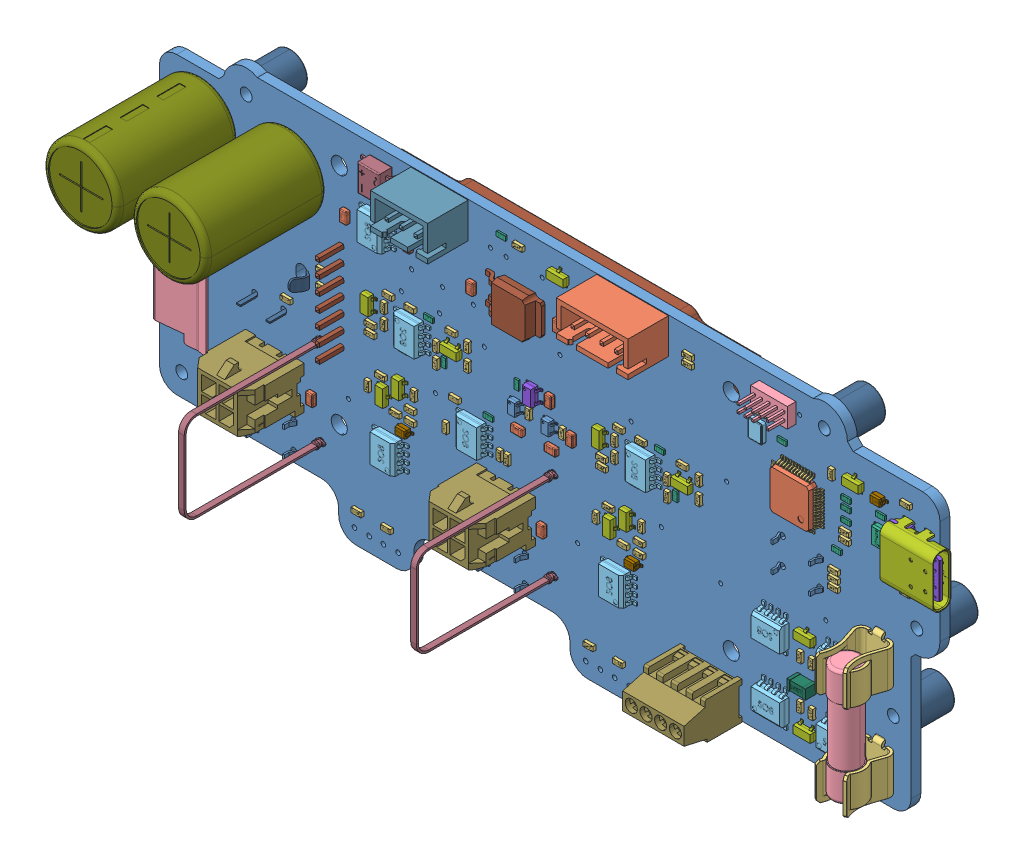
SolidWorks assembly SolderingStation, configuration Default. Lengths in mm.
Overall size (142.21 62 43.76).
390 component instances, 40 part files, 0 mates.
Components (placement in the parent):
- SolderingStation.step-1: SolderingStation.step [Default] at origin size (142.21 62 43.76)
  - Board_ss.step-1: Board_ss.step [Default] at origin size (140 62 1.69)
    - Open CASCADE STEP translator 6.8 4.1.1.step-1: Open CASCADE STEP translator 6.8 4.1.1.step [Default] at (0 0 -1.6914) size (140 62 1.69)
  - C17_ss.step-1: C17_ss.step [Default] at origin size (1.25 2 0.78)
    - User_Library-0805_SMD_Capacitor.step-1: User_Library-0805_SMD_Capacitor.step [Default] at (110.8455 64.7701 0) x (0 1 0) z (1 0 0) size (2 0.78 1.25)
  - R45_ss.step-1: R45_ss.step [Default] at origin size (1.7 0.8 0.56)
    - User_Library-RES_1609-0603.step-1: User_Library-RES_1609-0603.step [Default] at (65.2781 57.15 0) x (1 0 0) z (0 -1 0) size (1.7 0.56 0.8)
  - N1_ss.step-1: N1_ss.step [Default] at origin size (9.09 12.8 3.73)
    - nal-clip.step-1: nal-clip.step [Default] at (42.9877 48.2091 -0.8) x (0 0 -1) z (0 -1 0) size (3.73 9.09 12.8)
  - U2_ss.step-1: U2_ss.step [Default] at origin size (6.2 5 1.75)
    - User_Library-SOIC8_JEDEC_MS-012AA.step-1: User_Library-SOIC8_JEDEC_MS-012AA.step [Default] at (80.8676 75.6667 0) x (0 1 0) z (1 0 0) size (5 1.75 6.2)
  - C15_ss.step-1: C15_ss.step [Default] at origin size (1.6 0.8 0.3)
    - User_Library-0603_SMD_Capacitor.step-1: User_Library-0603_SMD_Capacitor.step [Default] at (161.9249 74.0409 0) x (-1 0 0) z (0 1 0) size (1.6 0.3 0.8)
  - C18_ss.step-1: C18_ss.step [Default] at origin size (1.6 0.8 0.3)
    - User_Library-0603_SMD_Capacitor.step-1: User_Library-0603_SMD_Capacitor.step [Default] at (161.9249 75.4379 0) x (-1 0 0) z (0 1 0) size (1.6 0.3 0.8)
  - U10_ss.step-1: U10_ss.step [Default] at origin size (3 2.5 1.1)
    - CircuitWorks-SOT-23.step-1: CircuitWorks-SOT-23.step [Default] at (163.4489 78.7147 0.5) x (-1 0 0) z (0 1 0) size (3 1.1 2.5)
  - U9_ss.step-1: U9_ss.step [Default] at origin size (2.8 2.9 1.45)
    - User_Library-SOT23-5-2.step-1: User_Library-SOT23-5-2.step [Default] at (107.9245 64.4143 0) x (0 -1 0) z (0 0 1) size (2.9 2.8 1.45)
  - C27_ss.step-1: C27_ss.step [Default] at origin size (1.25 2 0.78)
    - User_Library-0805_SMD_Capacitor.step-1: User_Library-0805_SMD_Capacitor.step [Default] at (114.5539 60.8331 0) x (0 1 0) z (1 0 0) size (2 0.78 1.25)
  - C26_ss.step-1: C26_ss.step [Default] at origin size (0.8 1.6 0.3)
    - User_Library-0603_SMD_Capacitor.step-1: User_Library-0603_SMD_Capacitor.step [Default] at (105.0035 64.1605 0) x (0 1 0) z (1 0 0) size (1.6 0.3 0.8)
  - C25_ss.step-1: C25_ss.step [Default] at origin size (1.25 2 0.78)
    - User_Library-0805_SMD_Capacitor.step-1: User_Library-0805_SMD_Capacitor.step [Default] at (109.4741 44.7039 0) x (0 -1 0) z (-1 0 0) size (2 0.78 1.25)
  - C24_ss.step-1: C24_ss.step [Default] at origin size (1.25 2 0.78)
    - User_Library-0805_SMD_Capacitor.step-1: User_Library-0805_SMD_Capacitor.step [Default] at (69.5961 44.4499 0) x (0 -1 0) z (-1 0 0) size (2 0.78 1.25)
  - D13_ss.step-1: D13_ss.step [Default] at origin size (2.7 1.25 1.1)
    - User_Library-SOD2513X11.step-1: User_Library-SOD2513X11.step [Default] at (167.7671 78.5115 0) x (1 0 0) z (0 0 1) size (2.7 1.25 1.1)
  - C22_ss.step-1: C22_ss.step [Default] at origin size (2 1.25 0.78)
    - User_Library-0805_SMD_Capacitor.step-1: User_Library-0805_SMD_Capacitor.step [Default] at (105.3871 57.6581 0) x (1 0 0) z (0 -1 0) size (2 0.78 1.25)
  - C23_ss.step-1: C23_ss.step [Default] at origin size (2 1.25 0.78)
    - User_Library-0805_SMD_Capacitor.step-1: User_Library-0805_SMD_Capacitor.step [Default] at (111.2291 57.6581 0) x (1 0 0) z (0 -1 0) size (2 0.78 1.25)
  - C21_ss.step-1: C21_ss.step [Default] at origin size (1.6 0.8 0.3)
    - User_Library-0603_SMD_Capacitor.step-1: User_Library-0603_SMD_Capacitor.step [Default] at (102.3367 85.0901 0) x (1 0 0) z (0 -1 0) size (1.6 0.3 0.8)
  - SP6_ss.step-1: SP6_ss.step [Default] at origin size (6 6 6)
    - 6mmSpacer.step-1: 6mmSpacer.step [Default] at (46.8629 36.8301 -1.6914) x (-1 0 0) z (0 -1 0) size (6 6 6)
  - SP5_ss.step-1: SP5_ss.step [Default] at origin size (6 6 6)
    - 6mmSpacer.step-1: 6mmSpacer.step [Default] at (169.9259 46.8631 -1.6914) x (-1 0 0) z (0 -1 0) size (6 6 6)
  - D2_ss.step-1: D2_ss.step [Default] at origin size (2.7 1.25 1.1)
    - User_Library-SOD2513X11.step-1: User_Library-SOD2513X11.step [Default] at (125.2719 47.6779 0) x (-1 0 0) z (0 0 1) size (2.7 1.25 1.1)
  - U1_ss.step-1: U1_ss.step [Default] at origin size (9.94 6.54 2.42)
    - User_Library-DPAK-1.step-1: User_Library-DPAK-1.step [Default] at (105.596 76.2 1.15) x (0 -1 0) z (-1 0 0) size (6.54 2.42 9.94)
  - C20_ss.step-1: C20_ss.step [Default] at origin size (0.8 1.6 0.3)
    - User_Library-0603_SMD_Capacitor.step-1: User_Library-0603_SMD_Capacitor.step [Default] at (132.4355 61.1887 0) x (0 1 0) z (1 0 0) size (1.6 0.3 0.8)
  - C7_ss.step-1: C7_ss.step [Default] at origin size (0.8 1.6 0.3)
    - User_Library-0603_SMD_Capacitor.step-1: User_Library-0603_SMD_Capacitor.step [Default] at (92.3797 61.1631 0) x (0 1 0) z (1 0 0) size (1.6 0.3 0.8)
  - P1_ss.step-1: P1_ss.step [Default] at origin size (10.62 6.5 13.4)
    - c-282834-4-c-3d.step-1: c-282834-4-c-3d.step [Default] at (138.4201 36.0681 10) size (10.62 6.5 13.4)
  - R25_ss.step-1: R25_ss.step [Default] at origin size (1.65 16.48 27.41)
    - OAR3.step-1: OAR3.step [Default] at (70.9931 46.1009 -3.2) x (0 -1 0) z (-1 0 0) size (16.48 27.41 1.65)
  - R26_ss.step-1: R26_ss.step [Default] at origin size (1.65 16.48 27.41)
    - OAR3.step-1: OAR3.step [Default] at (111.1505 46.1009 -3.2) x (0 -1 0) z (-1 0 0) size (16.48 27.41 1.65)
  - R19_ss.step-1: R19_ss.step [Default] at origin size (0.8 1.7 0.56)
    - User_Library-RES_1609-0603.step-1: User_Library-RES_1609-0603.step [Default] at (154.101 48.0431 0) x (0 1 0) z (1 0 0) size (1.7 0.56 0.8)
  - R20_ss.step-1: R20_ss.step [Default] at origin size (0.8 1.7 0.56)
    - User_Library-RES_1609-0603.step-1: User_Library-RES_1609-0603.step [Default] at (156.1329 48.0431 0) x (0 1 0) z (1 0 0) size (1.7 0.56 0.8)
  - R27_ss.step-1: R27_ss.step [Default] at origin size (0.8 1.7 0.56)
    - User_Library-RES_1609-0603.step-1: User_Library-RES_1609-0603.step [Default] at (154.101 40.5501 0) x (0 1 0) z (1 0 0) size (1.7 0.56 0.8)
  - R28_ss.step-1: R28_ss.step [Default] at origin size (0.8 1.7 0.56)
    - User_Library-RES_1609-0603.step-1: User_Library-RES_1609-0603.step [Default] at (156.1329 40.5501 0) x (0 1 0) z (1 0 0) size (1.7 0.56 0.8)
  - D11_ss.step-1: D11_ss.step [Default] at origin size (3.5 3.8 10)
    - Red-LED_3MM.step-1: Red-LED_3MM.step [Default] at (77.9999 28.5001 -5.6914) x (0 1 0) z (0 0 -1) size (3.8 3.5 10)
  - D9_ss.step-1: D9_ss.step [Default] at origin size (3.5 3.8 10)
    - Red-LED_3MM.step-1: Red-LED_3MM.step [Default] at (117.9999 28.5001 -5.6914) x (0 1 0) z (0 0 -1) size (3.8 3.5 10)
  - D10_ss.step-1: D10_ss.step [Default] at origin size (3.5 3.8 10)
    - Green-LED_3MM.step-1: Green-LED_3MM.step [Default] at (122.9999 28.5001 -5.6914) x (0 1 0) z (0 0 -1) size (3.8 3.5 10)
  - D12_ss.step-1: D12_ss.step [Default] at origin size (3.5 3.8 10)
    - Green-LED_3MM.step-1: Green-LED_3MM.step [Default] at (82.9999 28.5001 -5.6914) x (0 1 0) z (0 0 -1) size (3.8 3.5 10)
  - S2_ss.step-1: S2_ss.step [Default] at origin size (7.7 6 10.2)
    - User_Library-b3w1050.step-1: User_Library-b3w1050.step [Default] at (63 36.9999 -1.6914) x (1 0 0) z (0 1 0) size (3.5 1.6 3.5)
    - User_Library-b3w1050.step-2: User_Library-b3w1050.step [Default] at (63 36.9999 -1.6914) x (1 0 0) z (0 1 0) size (3.5 1.6 3.5)
    - User_Library-b3w1050-0.step-1: User_Library-b3w1050-0.step [Default] at (63 36.9999 -1.6914) x (1 0 0) z (0 1 0) size (3.5 1.6 3.5)
    - User_Library-b3w1050-1.step-1: User_Library-b3w1050-1.step [Default] at (63 36.9999 -1.6914) x (1 0 0) z (0 1 0) size (7.7 10.2 6)
    - User_Library-b3w1050-1.step-2: User_Library-b3w1050-1.step [Default] at (63 36.9999 -1.6914) x (1 0 0) z (0 1 0) size (7.7 10.2 6)
    - User_Library-b3w1050-2.step-1: User_Library-b3w1050-2.step [Default] at (63 36.9999 -1.6914) x (1 0 0) z (0 1 0) size (7.7 10.2 6)
  - S1_ss.step-1: S1_ss.step [Default] at origin size (7.7 6 10.2)
    - User_Library-b3w1050.step-1: User_Library-b3w1050.step [Default] at (154 62.0001 -1.6914) x (-1 0 0) z (0 -1 0) size (3.5 1.6 3.5)
    - User_Library-b3w1050.step-2: User_Library-b3w1050.step [Default] at (154 62.0001 -1.6914) x (-1 0 0) z (0 -1 0) size (3.5 1.6 3.5)
    - User_Library-b3w1050-0.step-1: User_Library-b3w1050-0.step [Default] at (154 62.0001 -1.6914) x (-1 0 0) z (0 -1 0) size (3.5 1.6 3.5)
    - User_Library-b3w1050-1.step-1: User_Library-b3w1050-1.step [Default] at (154 62.0001 -1.6914) x (-1 0 0) z (0 -1 0) size (7.7 10.2 6)
    - User_Library-b3w1050-1.step-2: User_Library-b3w1050-1.step [Default] at (154 62.0001 -1.6914) x (-1 0 0) z (0 -1 0) size (7.7 10.2 6)
    - User_Library-b3w1050-2.step-1: User_Library-b3w1050-2.step [Default] at (154 62.0001 -1.6914) x (-1 0 0) z (0 -1 0) size (7.7 10.2 6)
  - S3_ss.step-1: S3_ss.step [Default] at origin size (7.7 6 10.2)
    - User_Library-b3w1050.step-1: User_Library-b3w1050.step [Default] at (103 36.9999 -1.6914) x (1 0 0) z (0 1 0) size (3.5 1.6 3.5)
    - User_Library-b3w1050.step-2: User_Library-b3w1050.step [Default] at (103 36.9999 -1.6914) x (1 0 0) z (0 1 0) size (3.5 1.6 3.5)
    - User_Library-b3w1050-0.step-1: User_Library-b3w1050-0.step [Default] at (103 36.9999 -1.6914) x (1 0 0) z (0 1 0) size (3.5 1.6 3.5)
    - User_Library-b3w1050-1.step-1: User_Library-b3w1050-1.step [Default] at (103 36.9999 -1.6914) x (1 0 0) z (0 1 0) size (7.7 10.2 6)
    - User_Library-b3w1050-1.step-2: User_Library-b3w1050-1.step [Default] at (103 36.9999 -1.6914) x (1 0 0) z (0 1 0) size (7.7 10.2 6)
    - User_Library-b3w1050-2.step-1: User_Library-b3w1050-2.step [Default] at (103 36.9999 -1.6914) x (1 0 0) z (0 1 0) size (7.7 10.2 6)
  - U5_ss.step-1: U5_ss.step [Default] at origin size (9 9 1.6)
    - User_Library-LQFP48_Grid_0.5.step-1: User_Library-LQFP48_Grid_0.5.step [Default] at (153.5238 71.918 0) x (0 1 0) z (1 0 0) size (9 1.6 9)
      - User_Library-LQFP48_Grid_0.5_LQFP48_Koerper_2.step-1: User_Library-LQFP48_Grid_0.5_LQFP48_Koerper_2.step [Default] at origin size (7 1.45 7)
      - User_Library-LQFP48_Grid_0.5_LQFP_PIN_2.step-1: User_Library-LQFP48_Grid_0.5_LQFP_PIN_2.step [Default] at (-2.75 0 4.5) size (0.27 0.97 1.5)
      - User_Library-LQFP48_Grid_0.5_LQFP_PIN_2.step-2: User_Library-LQFP48_Grid_0.5_LQFP_PIN_2.step [Default] at (-2.25 0 4.5) size (0.27 0.97 1.5)
      - User_Library-LQFP48_Grid_0.5_LQFP_PIN_2.step-3: User_Library-LQFP48_Grid_0.5_LQFP_PIN_2.step [Default] at (-1.75 0 4.5) size (0.27 0.97 1.5)
      - User_Library-LQFP48_Grid_0.5_LQFP_PIN_2.step-4: User_Library-LQFP48_Grid_0.5_LQFP_PIN_2.step [Default] at (-1.25 0 4.5) size (0.27 0.97 1.5)
      - User_Library-LQFP48_Grid_0.5_LQFP_PIN_2.step-5: User_Library-LQFP48_Grid_0.5_LQFP_PIN_2.step [Default] at (-0.75 0 4.5) size (0.27 0.97 1.5)
      - User_Library-LQFP48_Grid_0.5_LQFP_PIN_2.step-6: User_Library-LQFP48_Grid_0.5_LQFP_PIN_2.step [Default] at (-0.25 0 4.5) size (0.27 0.97 1.5)
      - User_Library-LQFP48_Grid_0.5_LQFP_PIN_2.step-7: User_Library-LQFP48_Grid_0.5_LQFP_PIN_2.step [Default] at (0.25 0 4.5) size (0.27 0.97 1.5)
      - User_Library-LQFP48_Grid_0.5_LQFP_PIN_2.step-8: User_Library-LQFP48_Grid_0.5_LQFP_PIN_2.step [Default] at (0.75 0 4.5) size (0.27 0.97 1.5)
      - User_Library-LQFP48_Grid_0.5_LQFP_PIN_2.step-9: User_Library-LQFP48_Grid_0.5_LQFP_PIN_2.step [Default] at (1.25 0 4.5) size (0.27 0.97 1.5)
      - User_Library-LQFP48_Grid_0.5_LQFP_PIN_2.step-10: User_Library-LQFP48_Grid_0.5_LQFP_PIN_2.step [Default] at (1.75 0 4.5) size (0.27 0.97 1.5)
      - User_Library-LQFP48_Grid_0.5_LQFP_PIN_2.step-11: User_Library-LQFP48_Grid_0.5_LQFP_PIN_2.step [Default] at (2.25 0 4.5) size (0.27 0.97 1.5)
      - User_Library-LQFP48_Grid_0.5_LQFP_PIN_2.step-12: User_Library-LQFP48_Grid_0.5_LQFP_PIN_2.step [Default] at (2.75 0 4.5) size (0.27 0.97 1.5)
      - User_Library-LQFP48_Grid_0.5_LQFP_PIN_2.step-13: User_Library-LQFP48_Grid_0.5_LQFP_PIN_2.step [Default] at (4.5 0 2.75) x (0 0 -1) z (1 0 0) size (0.27 0.97 1.5)
      - User_Library-LQFP48_Grid_0.5_LQFP_PIN_2.step-14: User_Library-LQFP48_Grid_0.5_LQFP_PIN_2.step [Default] at (4.5 0 2.25) x (0 0 -1) z (1 0 0) size (0.27 0.97 1.5)
      - User_Library-LQFP48_Grid_0.5_LQFP_PIN_2.step-15: User_Library-LQFP48_Grid_0.5_LQFP_PIN_2.step [Default] at (4.5 0 1.75) x (0 0 -1) z (1 0 0) size (0.27 0.97 1.5)
      - User_Library-LQFP48_Grid_0.5_LQFP_PIN_2.step-16: User_Library-LQFP48_Grid_0.5_LQFP_PIN_2.step [Default] at (4.5 0 1.25) x (0 0 -1) z (1 0 0) size (0.27 0.97 1.5)
      - User_Library-LQFP48_Grid_0.5_LQFP_PIN_2.step-17: User_Library-LQFP48_Grid_0.5_LQFP_PIN_2.step [Default] at (4.5 0 0.75) x (0 0 -1) z (1 0 0) size (0.27 0.97 1.5)
      - User_Library-LQFP48_Grid_0.5_LQFP_PIN_2.step-18: User_Library-LQFP48_Grid_0.5_LQFP_PIN_2.step [Default] at (4.5 0 0.25) x (0 0 -1) z (1 0 0) size (0.27 0.97 1.5)
      - User_Library-LQFP48_Grid_0.5_LQFP_PIN_2.step-19: User_Library-LQFP48_Grid_0.5_LQFP_PIN_2.step [Default] at (4.5 0 -0.25) x (0 0 -1) z (1 0 0) size (0.27 0.97 1.5)
      - User_Library-LQFP48_Grid_0.5_LQFP_PIN_2.step-20: User_Library-LQFP48_Grid_0.5_LQFP_PIN_2.step [Default] at (4.5 0 -0.75) x (0 0 -1) z (1 0 0) size (0.27 0.97 1.5)
      - User_Library-LQFP48_Grid_0.5_LQFP_PIN_2.step-21: User_Library-LQFP48_Grid_0.5_LQFP_PIN_2.step [Default] at (4.5 0 -1.25) x (0 0 -1) z (1 0 0) size (0.27 0.97 1.5)
      - User_Library-LQFP48_Grid_0.5_LQFP_PIN_2.step-22: User_Library-LQFP48_Grid_0.5_LQFP_PIN_2.step [Default] at (4.5 0 -1.75) x (0 0 -1) z (1 0 0) size (0.27 0.97 1.5)
      - User_Library-LQFP48_Grid_0.5_LQFP_PIN_2.step-23: User_Library-LQFP48_Grid_0.5_LQFP_PIN_2.step [Default] at (4.5 0 -2.25) x (0 0 -1) z (1 0 0) size (0.27 0.97 1.5)
      - User_Library-LQFP48_Grid_0.5_LQFP_PIN_2.step-24: User_Library-LQFP48_Grid_0.5_LQFP_PIN_2.step [Default] at (4.5 0 -2.75) x (0 0 -1) z (1 0 0) size (0.27 0.97 1.5)
      - User_Library-LQFP48_Grid_0.5_LQFP_PIN_2.step-25: User_Library-LQFP48_Grid_0.5_LQFP_PIN_2.step [Default] at (2.75 0 -4.5) x (-1 0 0) z (0 0 -1) size (0.27 0.97 1.5)
      - User_Library-LQFP48_Grid_0.5_LQFP_PIN_2.step-26: User_Library-LQFP48_Grid_0.5_LQFP_PIN_2.step [Default] at (2.25 0 -4.5) x (-1 0 0) z (0 0 -1) size (0.27 0.97 1.5)
      - User_Library-LQFP48_Grid_0.5_LQFP_PIN_2.step-27: User_Library-LQFP48_Grid_0.5_LQFP_PIN_2.step [Default] at (1.75 0 -4.5) x (-1 0 0) z (0 0 -1) size (0.27 0.97 1.5)
      - User_Library-LQFP48_Grid_0.5_LQFP_PIN_2.step-28: User_Library-LQFP48_Grid_0.5_LQFP_PIN_2.step [Default] at (1.25 0 -4.5) x (-1 0 0) z (0 0 -1) size (0.27 0.97 1.5)
      - User_Library-LQFP48_Grid_0.5_LQFP_PIN_2.step-29: User_Library-LQFP48_Grid_0.5_LQFP_PIN_2.step [Default] at (0.75 0 -4.5) x (-1 0 0) z (0 0 -1) size (0.27 0.97 1.5)
      - User_Library-LQFP48_Grid_0.5_LQFP_PIN_2.step-30: User_Library-LQFP48_Grid_0.5_LQFP_PIN_2.step [Default] at (0.25 0 -4.5) x (-1 0 0) z (0 0 -1) size (0.27 0.97 1.5)
      - User_Library-LQFP48_Grid_0.5_LQFP_PIN_2.step-31: User_Library-LQFP48_Grid_0.5_LQFP_PIN_2.step [Default] at (-0.25 0 -4.5) x (-1 0 0) z (0 0 -1) size (0.27 0.97 1.5)
      - User_Library-LQFP48_Grid_0.5_LQFP_PIN_2.step-32: User_Library-LQFP48_Grid_0.5_LQFP_PIN_2.step [Default] at (-0.75 0 -4.5) x (-1 0 0) z (0 0 -1) size (0.27 0.97 1.5)
      - User_Library-LQFP48_Grid_0.5_LQFP_PIN_2.step-33: User_Library-LQFP48_Grid_0.5_LQFP_PIN_2.step [Default] at (-1.25 0 -4.5) x (-1 0 0) z (0 0 -1) size (0.27 0.97 1.5)
      - User_Library-LQFP48_Grid_0.5_LQFP_PIN_2.step-34: User_Library-LQFP48_Grid_0.5_LQFP_PIN_2.step [Default] at (-1.75 0 -4.5) x (-1 0 0) z (0 0 -1) size (0.27 0.97 1.5)
      - User_Library-LQFP48_Grid_0.5_LQFP_PIN_2.step-35: User_Library-LQFP48_Grid_0.5_LQFP_PIN_2.step [Default] at (-2.25 0 -4.5) x (-1 0 0) z (0 0 -1) size (0.27 0.97 1.5)
      - User_Library-LQFP48_Grid_0.5_LQFP_PIN_2.step-36: User_Library-LQFP48_Grid_0.5_LQFP_PIN_2.step [Default] at (-2.75 0 -4.5) x (-1 0 0) z (0 0 -1) size (0.27 0.97 1.5)
      - User_Library-LQFP48_Grid_0.5_LQFP_PIN_2.step-37: User_Library-LQFP48_Grid_0.5_LQFP_PIN_2.step [Default] at (-4.5 0 -2.75) x (0 0 1) z (-1 0 0) size (0.27 0.97 1.5)
      - User_Library-LQFP48_Grid_0.5_LQFP_PIN_2.step-38: User_Library-LQFP48_Grid_0.5_LQFP_PIN_2.step [Default] at (-4.5 0 -2.25) x (0 0 1) z (-1 0 0) size (0.27 0.97 1.5)
      - User_Library-LQFP48_Grid_0.5_LQFP_PIN_2.step-39: User_Library-LQFP48_Grid_0.5_LQFP_PIN_2.step [Default] at (-4.5 0 -1.75) x (0 0 1) z (-1 0 0) size (0.27 0.97 1.5)
      - User_Library-LQFP48_Grid_0.5_LQFP_PIN_2.step-40: User_Library-LQFP48_Grid_0.5_LQFP_PIN_2.step [Default] at (-4.5 0 -1.25) x (0 0 1) z (-1 0 0) size (0.27 0.97 1.5)
      - User_Library-LQFP48_Grid_0.5_LQFP_PIN_2.step-41: User_Library-LQFP48_Grid_0.5_LQFP_PIN_2.step [Default] at (-4.5 0 -0.75) x (0 0 1) z (-1 0 0) size (0.27 0.97 1.5)
      - User_Library-LQFP48_Grid_0.5_LQFP_PIN_2.step-42: User_Library-LQFP48_Grid_0.5_LQFP_PIN_2.step [Default] at (-4.5 0 -0.25) x (0 0 1) z (-1 0 0) size (0.27 0.97 1.5)
      - User_Library-LQFP48_Grid_0.5_LQFP_PIN_2.step-43: User_Library-LQFP48_Grid_0.5_LQFP_PIN_2.step [Default] at (-4.5 0 0.25) x (0 0 1) z (-1 0 0) size (0.27 0.97 1.5)
      - User_Library-LQFP48_Grid_0.5_LQFP_PIN_2.step-44: User_Library-LQFP48_Grid_0.5_LQFP_PIN_2.step [Default] at (-4.5 0 0.75) x (0 0 1) z (-1 0 0) size (0.27 0.97 1.5)
      - User_Library-LQFP48_Grid_0.5_LQFP_PIN_2.step-45: User_Library-LQFP48_Grid_0.5_LQFP_PIN_2.step [Default] at (-4.5 0 1.25) x (0 0 1) z (-1 0 0) size (0.27 0.97 1.5)
      - User_Library-LQFP48_Grid_0.5_LQFP_PIN_2.step-46: User_Library-LQFP48_Grid_0.5_LQFP_PIN_2.step [Default] at (-4.5 0 1.75) x (0 0 1) z (-1 0 0) size (0.27 0.97 1.5)
      - User_Library-LQFP48_Grid_0.5_LQFP_PIN_2.step-47: User_Library-LQFP48_Grid_0.5_LQFP_PIN_2.step [Default] at (-4.5 0 2.25) x (0 0 1) z (-1 0 0) size (0.27 0.97 1.5)
      - User_Library-LQFP48_Grid_0.5_LQFP_PIN_2.step-48: User_Library-LQFP48_Grid_0.5_LQFP_PIN_2.step [Default] at (-4.5 0 2.75) x (0 0 1) z (-1 0 0) size (0.27 0.97 1.5)
  - C12_ss.step-1: C12_ss.step [Default] at origin size (1.6 0.8 0.3)
    - User_Library-0603_SMD_Capacitor.step-1: User_Library-0603_SMD_Capacitor.step [Default] at (167.9195 75.9461 0) x (1 0 0) z (0 -1 0) size (1.6 0.3 0.8)
  - C13_ss.step-1: C13_ss.step [Default] at origin size (1.6 0.8 0.3)
    - User_Library-0603_SMD_Capacitor.step-1: User_Library-0603_SMD_Capacitor.step [Default] at (161.9249 72.1359 0) x (-1 0 0) z (0 1 0) size (1.6 0.3 0.8)
  - C14_ss.step-1: C14_ss.step [Default] at origin size (1.6 0.8 0.3)
    - User_Library-0603_SMD_Capacitor.step-1: User_Library-0603_SMD_Capacitor.step [Default] at (150.8761 78.6131 0) x (1 0 0) z (0 -1 0) size (1.6 0.3 0.8)
  - C16_ss.step-1: C16_ss.step [Default] at origin size (1.6 0.8 0.3)
    - User_Library-0603_SMD_Capacitor.step-1: User_Library-0603_SMD_Capacitor.step [Default] at (160.3239 66.9819 0) x (-1 0 0) z (0 1 0) size (1.6 0.3 0.8)
  - P6_ss.step-1: P6_ss.step [Default] at origin size (6.35 3.4 6.8)
    - SWD2x5.step-1: SWD2x5.step [Default] at (153.0859 83.8493 0) x (1 0 0) z (0 -1 0) size (6.35 6.8 3.4)
  - R38_ss.step-1: R38_ss.step [Default] at origin size (1.7 0.8 0.56)
    - User_Library-RES_1609-0603.step-1: User_Library-RES_1609-0603.step [Default] at (159.9431 62.537 0) x (1 0 0) z (0 -1 0) size (1.7 0.56 0.8)
  - R37_ss.step-1: R37_ss.step [Default] at origin size (1.7 0.8 0.56)
    - User_Library-RES_1609-0603.step-1: User_Library-RES_1609-0603.step [Default] at (159.9431 63.807 0) x (1 0 0) z (0 -1 0) size (1.7 0.56 0.8)
  - R40_ss.step-1: R40_ss.step [Default] at origin size (1.7 0.8 0.56)
    - User_Library-RES_1609-0603.step-1: User_Library-RES_1609-0603.step [Default] at (159.9431 61.267 0) x (1 0 0) z (0 -1 0) size (1.7 0.56 0.8)
  - R39_ss.step-1: R39_ss.step [Default] at origin size (1.7 0.8 0.56)
    - User_Library-RES_1609-0603.step-1: User_Library-RES_1609-0603.step [Default] at (172.3891 66.7281 0) x (1 0 0) z (0 -1 0) size (1.7 0.56 0.8)
  - R41_ss.step-1: R41_ss.step [Default] at origin size (1.7 0.8 0.56)
    - User_Library-RES_1609-0603.step-1: User_Library-RES_1609-0603.step [Default] at (172.3889 79.936 0) x (-1 0 0) z (0 1 0) size (1.7 0.56 0.8)
  - R42_ss.step-1: R42_ss.step [Default] at origin size (1.7 0.8 0.56)
    - User_Library-RES_1609-0603.step-1: User_Library-RES_1609-0603.step [Default] at (161.8479 70.5379 0) x (-1 0 0) z (0 1 0) size (1.7 0.56 0.8)
  - R43_ss.step-1: R43_ss.step [Default] at origin size (1.7 0.8 0.56)
    - User_Library-RES_1609-0603.step-1: User_Library-RES_1609-0603.step [Default] at (161.8479 69.268 0) x (-1 0 0) z (0 1 0) size (1.7 0.56 0.8)
  - R50_ss.step-1: R50_ss.step [Default] at origin size (1.7 0.8 0.56)
    - User_Library-RES_1609-0603.step-1: User_Library-RES_1609-0603.step [Default] at (77.5201 31.406 0) x (1 0 0) z (0 -1 0) size (1.7 0.56 0.8)
  - R47_ss.step-1: R47_ss.step [Default] at origin size (1.7 0.8 0.56)
    - User_Library-RES_1609-0603.step-1: User_Library-RES_1609-0603.step [Default] at (117.6519 31.422 0) x (-1 0 0) z (0 1 0) size (1.7 0.56 0.8)
  - R49_ss.step-1: R49_ss.step [Default] at origin size (1.7 0.8 0.56)
    - User_Library-RES_1609-0603.step-1: User_Library-RES_1609-0603.step [Default] at (122.7321 31.422 0) x (1 0 0) z (0 -1 0) size (1.7 0.56 0.8)
  - R52_ss.step-1: R52_ss.step [Default] at origin size (1.7 0.8 0.56)
    - User_Library-RES_1609-0603.step-1: User_Library-RES_1609-0603.step [Default] at (82.6001 31.406 0) x (1 0 0) z (0 -1 0) size (1.7 0.56 0.8)
  - R51_ss.step-1: R51_ss.step [Default] at origin size (1.7 0.8 0.56)
    - User_Library-RES_1609-0603.step-1: User_Library-RES_1609-0603.step [Default] at (71.3999 62 0) x (-1 0 0) z (0 1 0) size (1.7 0.56 0.8)
  - R53_ss.step-1: R53_ss.step [Default] at origin size (1.7 0.8 0.56)
    - User_Library-RES_1609-0603.step-1: User_Library-RES_1609-0603.step [Default] at (71.3999 64.5 0) x (-1 0 0) z (0 1 0) size (1.7 0.56 0.8)
  - Y1_ss.step-1: Y1_ss.step [Default] at origin size (2.5 3.2 0.7)
    - EPSON-FA-238.step-1: EPSON-FA-238.step [Default] at (146.624 78.2189 0) x (0 1 0) z (1 0 0) size (3.2 0.7 2.5)
  - Z1_ss.step-1: Z1_ss.step [Default] at origin size (2.84 2.9 1.28)
    - SOT-23-6_(SOT457,SC-74).step-1: SOT-23-6_(SOT457,SC-74).step [Default] at (167.3089 71.8081 0.1) x (1 0 0) z (0 -1 0) size (2.84 1.28 2.9)
  - Q9_ss.step-1: Q9_ss.step [Default] at origin size (5 6.2 1.75)
    - User_Library-SOIC8_JEDEC_MS-012AA.step-1: User_Library-SOIC8_JEDEC_MS-012AA.step [Default] at (160.7051 38.7721 0) x (1 0 0) z (0 -1 0) size (5 1.75 6.2)
  - Q10_ss.step-1: Q10_ss.step [Default] at origin size (5 6.2 1.75)
    - User_Library-SOIC8_JEDEC_MS-012AA.step-1: User_Library-SOIC8_JEDEC_MS-012AA.step [Default] at (149.5291 38.7721 0) x (1 0 0) z (0 -1 0) size (5 1.75 6.2)
  - Q8_ss.step-1: Q8_ss.step [Default] at origin size (5 6.2 1.75)
    - User_Library-SOIC8_JEDEC_MS-012AA.step-1: User_Library-SOIC8_JEDEC_MS-012AA.step [Default] at (160.7049 49.9479 0) x (-1 0 0) z (0 1 0) size (5 1.75 6.2)
  - Q7_ss.step-1: Q7_ss.step [Default] at origin size (5 6.2 1.75)
    - User_Library-SOIC8_JEDEC_MS-012AA.step-1: User_Library-SOIC8_JEDEC_MS-012AA.step [Default] at (149.5289 49.9479 0) x (-1 0 0) z (0 1 0) size (5 1.75 6.2)
  - D6_ss.step-1: D6_ss.step [Default] at origin size (3 2.5 1.1)
    - CircuitWorks-SOT-23.step-1: CircuitWorks-SOT-23.step [Default] at (155.1171 37.2479 0.5) x (1 0 0) z (0 -1 0) size (3 1.1 2.5)
  - D5_ss.step-1: D5_ss.step [Default] at origin size (3 2.5 1.1)
    - CircuitWorks-SOT-23.step-1: CircuitWorks-SOT-23.step [Default] at (155.1169 51.472 0.5) x (-1 0 0) z (0 1 0) size (3 1.1 2.5)
  - USB1_ss.step-1: USB1_ss.step [Default] at origin size (9.17 9.03 5.56)
    - USB4085-03-A_revA.step-1: USB4085-03-A_revA.step [Default] at (179.7088 73.2001 0) x (0 1 0) z (1 0 0) size (9.03 5.56 9.17)
      - shell_1___.step-1: shell_1___.step [Default] at origin size (8.96 5.56 9.15)
      - housing_1___.step-1: housing_1___.step [Default] at (0 3.15 0) x (1 0 0) z (0 1 0) size (9.03 9.07 4.75)
  - SC2_ss.step-1: SC2_ss.step [Default] at origin size (6 6 5.5)
    - Switch-Cap_-_b32-2000.step-1: Switch-Cap_-_b32-2000.step [Default] at (62.9999 37.0001 -6.1914) x (-1 0 0) z (0 -1 0) size (6 5.5 6)
  - SC3_ss.step-1: SC3_ss.step [Default] at origin size (6 6 5.5)
    - Switch-Cap_-_b32-2000.step-1: Switch-Cap_-_b32-2000.step [Default] at (102.9999 37.0001 -6.1914) x (-1 0 0) z (0 -1 0) size (6 5.5 6)
  - SC1_ss.step-1: SC1_ss.step [Default] at origin size (6 6 5.5)
    - Switch-Cap_-_b32-2000.step-1: Switch-Cap_-_b32-2000.step [Default] at (153.9999 62.0001 -6.1914) x (-1 0 0) z (0 -1 0) size (6 5.5 6)
  - E1_ss.step-1: E1_ss.step [Default] at origin size (15.01 15 22.55)
    - RotaryEncoder.step-1: RotaryEncoder.step [Default] at (62.0001 61.9999 -7.8414) x (1 0 0) z (0 -1 0) size (15.01 22.55 15)
  - OLED1_ss.step-1: OLED1_ss.step [Default] at origin size (72 43 12.5)
    - OLED_128x64_2-42inch.step-1: OLED_128x64_2-42inch.step [Default] at (108.0081 61.9493 -4.1914) x (1 0 0) z (0 1 0) size (72 12.5 43)
  - P2_ss.step-1: P2_ss.step [Default] at origin size (10.15 8.77 13.09)
    - 430450412.step-1: 430450412.step [Default] at (63.0001 45.397 5) x (1 0 0) z (0 0 1) size (10.15 8.77 13.09)
  - P3_ss.step-1: P3_ss.step [Default] at origin size (10.15 8.77 13.09)
    - 430450412.step-1: 430450412.step [Default] at (103.0001 45.397 5) x (1 0 0) z (0 0 1) size (10.15 8.77 13.09)
  - Q1_ss.step-1: Q1_ss.step [Default] at origin size (6.2 5 1.75)
    - User_Library-SOIC8_JEDEC_MS-012AA.step-1: User_Library-SOIC8_JEDEC_MS-012AA.step [Default] at (83.1079 43.4711 0) x (0 1 0) z (1 0 0) size (5 1.75 6.2)
  - R5_ss.step-1: R5_ss.step [Default] at origin size (1.7 0.8 0.56)
    - User_Library-RES_1609-0603.step-1: User_Library-RES_1609-0603.step [Default] at (84.1241 49.456 0) x (1 0 0) z (0 -1 0) size (1.7 0.56 0.8)
  - SP1_ss.step-1: SP1_ss.step [Default] at origin size (6 6 6)
    - 6mmSpacer.step-1: 6mmSpacer.step [Default] at (57.9999 84.0001 -1.6914) x (-1 0 0) z (0 -1 0) size (6 6 6)
  - SP2_ss.step-1: SP2_ss.step [Default] at origin size (6 6 6)
    - 6mmSpacer.step-1: 6mmSpacer.step [Default] at (41.9999 62.0001 -1.6914) x (-1 0 0) z (0 -1 0) size (6 6 6)
  - SP3_ss.step-1: SP3_ss.step [Default] at origin size (6 6 6)
    - 6mmSpacer.step-1: 6mmSpacer.step [Default] at (173.9999 62.0001 -1.6914) x (-1 0 0) z (0 -1 0) size (6 6 6)
  - SP4_ss.step-1: SP4_ss.step [Default] at origin size (6 6 6)
    - 6mmSpacer.step-1: 6mmSpacer.step [Default] at (157.9999 84.0001 -1.6914) x (-1 0 0) z (0 -1 0) size (6 6 6)
  - BR1_ss.step-1: BR1_ss.step [Default] at origin size (7 4.7 2.4)
    - FullWaveRectifier.step-1: FullWaveRectifier.step [Default] at (81.5339 83.5661 0.1) x (0 1 0) z (1 0 0) size (4.7 2.4 7)
  - C2_ss.step-1: C2_ss.step [Default] at origin size (1.25 2 0.78)
    - User_Library-0805_SMD_Capacitor.step-1: User_Library-0805_SMD_Capacitor.step [Default] at (112.2681 76.7079 0) x (0 -1 0) z (-1 0 0) size (2 0.78 1.25)
  - J2_ss.step-1: J2_ss.step [Default] at origin size (9.9 6.1 10.4)
    - User_Library-XH-A-3.step-1: User_Library-XH-A-3.step [Default] at (96.3901 87.3751 7) x (-1 0 0) z (0 0 1) size (9.9 6.1 10.4)
  - R1_ss.step-1: R1_ss.step [Default] at origin size (1.7 0.8 0.56)
    - User_Library-RES_1609-0603.step-1: User_Library-RES_1609-0603.step [Default] at (86.6641 49.456 0) x (1 0 0) z (0 -1 0) size (1.7 0.56 0.8)
  - RV1_ss.step-1: RV1_ss.step [Default] at origin size (3.2 1.7 1.9)
    - Varistor-1206.step-1: Varistor-1206.step [Default] at (154.9645 44.2997 0.01) x (-1 0 0) z (0 1 0) size (3.2 1.9 1.7)
  - C1_ss.step-1: C1_ss.step [Default] at origin size (1.25 2 0.78)
    - User_Library-0805_SMD_Capacitor.step-1: User_Library-0805_SMD_Capacitor.step [Default] at (97.2821 74.9299 0) x (0 -1 0) z (-1 0 0) size (2 0.78 1.25)
  - C5_ss.step-1: C5_ss.step [Default] at origin size (1.25 2 0.78)
    - User_Library-0805_SMD_Capacitor.step-1: User_Library-0805_SMD_Capacitor.step [Default] at (75.4379 74.7015 0) x (0 1 0) z (1 0 0) size (2 0.78 1.25)
  - C6_ss.step-1: C6_ss.step [Default] at origin size (1.25 2 0.78)
    - User_Library-0805_SMD_Capacitor.step-1: User_Library-0805_SMD_Capacitor.step [Default] at (86.3601 75.8189 0) x (0 -1 0) z (-1 0 0) size (2 0.78 1.25)
  - C3_ss.step-1: C3_ss.step [Default] at origin size (13 13 23.8)
    - RB5-13x21.step-1: RB5-13x21.step [Default] at (65.5321 76.7079 0) x (0 -1 0) z (-1 0 0) size (13 23.8 13)
  - C4_ss.step-1: C4_ss.step [Default] at origin size (13 13 23.8)
    - RB5-13x21.step-1: RB5-13x21.step [Default] at (50.2919 76.7081 0) x (0 1 0) z (1 0 0) size (13 23.8 13)
  - D1_ss.step-1: D1_ss.step [Default] at origin size (2.7 1.25 1.1)
    - User_Library-SOD2513X11.step-1: User_Library-SOD2513X11.step [Default] at (85.6479 47.6779 0) x (-1 0 0) z (0 0 1) size (2.7 1.25 1.1)
  - R48_ss.step-1: R48_ss.step [Default] at origin size (0.8 1.7 0.56)
    - User_Library-RES_1609-0603.step-1: User_Library-RES_1609-0603.step [Default] at (159.5121 78.1049 0) x (0 -1 0) z (-1 0 0) size (1.7 0.56 0.8)
  - R3_ss.step-1: R3_ss.step [Default] at origin size (0.8 1.7 0.56)
    - User_Library-RES_1609-0603.step-1: User_Library-RES_1609-0603.step [Default] at (87.299 53.7739 0) x (0 -1 0) z (-1 0 0) size (1.7 0.56 0.8)
  - R2_ss.step-1: R2_ss.step [Default] at origin size (1.7 0.8 0.56)
    - User_Library-RES_1609-0603.step-1: User_Library-RES_1609-0603.step [Default] at (126.2881 49.456 0) x (1 0 0) z (0 -1 0) size (1.7 0.56 0.8)
  - Q2_ss.step-1: Q2_ss.step [Default] at origin size (6.2 5 1.75)
    - User_Library-SOIC8_JEDEC_MS-012AA.step-1: User_Library-SOIC8_JEDEC_MS-012AA.step [Default] at (122.6199 43.4711 0) x (0 1 0) z (1 0 0) size (5 1.75 6.2)
  - Q4_ss.step-1: Q4_ss.step [Default] at origin size (2.5 3 1.1)
    - CircuitWorks-SOT-23.step-1: CircuitWorks-SOT-23.step [Default] at (124.129 53.7739 0.5) x (0 -1 0) z (-1 0 0) size (3 1.1 2.5)
  - Q5_ss.step-1: Q5_ss.step [Default] at origin size (2.5 3 1.1)
    - CircuitWorks-SOT-23.step-1: CircuitWorks-SOT-23.step [Default] at (81.965 51.2341 0.5) x (0 1 0) z (1 0 0) size (3 1.1 2.5)
  - Q6_ss.step-1: Q6_ss.step [Default] at origin size (2.5 3 1.1)
    - CircuitWorks-SOT-23.step-1: CircuitWorks-SOT-23.step [Default] at (121.3351 51.2341 0.5) x (0 1 0) z (1 0 0) size (3 1.1 2.5)
  - R4_ss.step-1: R4_ss.step [Default] at origin size (0.8 1.7 0.56)
    - User_Library-RES_1609-0603.step-1: User_Library-RES_1609-0603.step [Default] at (126.669 53.7739 0) x (0 -1 0) z (-1 0 0) size (1.7 0.56 0.8)
  - R6_ss.step-1: R6_ss.step [Default] at origin size (1.7 0.8 0.56)
    - User_Library-RES_1609-0603.step-1: User_Library-RES_1609-0603.step [Default] at (123.4941 49.456 0) x (1 0 0) z (0 -1 0) size (1.7 0.56 0.8)
  - R7_ss.step-1: R7_ss.step [Default] at origin size (1.7 0.8 0.56)
    - User_Library-RES_1609-0603.step-1: User_Library-RES_1609-0603.step [Default] at (86.6641 51.234 0) x (1 0 0) z (0 -1 0) size (1.7 0.56 0.8)
  - R8_ss.step-1: R8_ss.step [Default] at origin size (1.7 0.8 0.56)
    - User_Library-RES_1609-0603.step-1: User_Library-RES_1609-0603.step [Default] at (126.2881 51.234 0) x (1 0 0) z (0 -1 0) size (1.7 0.56 0.8)
  - R9_ss.step-1: R9_ss.step [Default] at origin size (1.7 0.8 0.56)
    - User_Library-RES_1609-0603.step-1: User_Library-RES_1609-0603.step [Default] at (81.5841 53.774 0) x (1 0 0) z (0 -1 0) size (1.7 0.56 0.8)
  - R10_ss.step-1: R10_ss.step [Default] at origin size (1.7 0.8 0.56)
    - User_Library-RES_1609-0603.step-1: User_Library-RES_1609-0603.step [Default] at (120.9541 53.774 0) x (1 0 0) z (0 -1 0) size (1.7 0.56 0.8)
  - R11_ss.step-1: R11_ss.step [Default] at origin size (0.8 1.7 0.56)
    - User_Library-RES_1609-0603.step-1: User_Library-RES_1609-0603.step [Default] at (79.298 51.2339 0) x (0 -1 0) z (-1 0 0) size (1.7 0.56 0.8)
  - R12_ss.step-1: R12_ss.step [Default] at origin size (0.8 1.7 0.56)
    - User_Library-RES_1609-0603.step-1: User_Library-RES_1609-0603.step [Default] at (118.7951 51.2339 0) x (0 -1 0) z (-1 0 0) size (1.7 0.56 0.8)
  - U3_ss.step-1: U3_ss.step [Default] at origin size (6.2 5 1.75)
    - User_Library-SOIC8_JEDEC_MS-012AA.step-1: User_Library-SOIC8_JEDEC_MS-012AA.step [Default] at (86.8348 63.0449 0) x (0 -1 0) z (-1 0 0) size (5 1.75 6.2)
  - C8_ss.step-1: C8_ss.step [Default] at origin size (1.6 0.8 0.3)
    - User_Library-0603_SMD_Capacitor.step-1: User_Library-0603_SMD_Capacitor.step [Default] at (89.7629 66.4487 0) x (1 0 0) z (0 -1 0) size (1.6 0.3 0.8)
  - C10_ss.step-1: C10_ss.step [Default] at origin size (1.6 0.8 0.3)
    - User_Library-0603_SMD_Capacitor.step-1: User_Library-0603_SMD_Capacitor.step [Default] at (85.2671 59.4891 0) x (1 0 0) z (0 -1 0) size (1.6 0.3 0.8)
  - D7_ss.step-1: D7_ss.step [Default] at origin size (2.5 3 1.1)
    - CircuitWorks-SOT-23.step-1: CircuitWorks-SOT-23.step [Default] at (79.4249 63.6799 0.5) x (0 -1 0) z (-1 0 0) size (3 1.1 2.5)
  - D3_ss.step-1: D3_ss.step [Default] at origin size (3 2.5 1.1)
    - CircuitWorks-SOT-23.step-1: CircuitWorks-SOT-23.step [Default] at (93.9031 63.8069 0.5) x (1 0 0) z (0 -1 0) size (3 1.1 2.5)
  - R13_ss.step-1: R13_ss.step [Default] at origin size (1.7 0.8 0.56)
    - User_Library-RES_1609-0603.step-1: User_Library-RES_1609-0603.step [Default] at (93.7759 66.474 0) x (-1 0 0) z (0 1 0) size (1.7 0.56 0.8)
  - R15_ss.step-1: R15_ss.step [Default] at origin size (0.8 1.7 0.56)
    - User_Library-RES_1609-0603.step-1: User_Library-RES_1609-0603.step [Default] at (96.57 65.7121 0) x (0 1 0) z (1 0 0) size (1.7 0.56 0.8)
  - R17_ss.step-1: R17_ss.step [Default] at origin size (0.8 1.7 0.56)
    - User_Library-RES_1609-0603.step-1: User_Library-RES_1609-0603.step [Default] at (96.57 62.7911 0) x (0 1 0) z (1 0 0) size (1.7 0.56 0.8)
  - R21_ss.step-1: R21_ss.step [Default] at origin size (0.8 1.7 0.56)
    - User_Library-RES_1609-0603.step-1: User_Library-RES_1609-0603.step [Default] at (91.1352 60.5051 0) x (0 1 0) z (1 0 0) size (1.7 0.56 0.8)
  - R22_ss.step-1: R22_ss.step [Default] at origin size (0.8 1.7 0.56)
    - User_Library-RES_1609-0603.step-1: User_Library-RES_1609-0603.step [Default] at (91.1352 63.0451 0) x (0 1 0) z (1 0 0) size (1.7 0.56 0.8)
  - R29_ss.step-1: R29_ss.step [Default] at origin size (1.7 0.8 0.56)
    - User_Library-RES_1609-0603.step-1: User_Library-RES_1609-0603.step [Default] at (79.8061 59.235 0) x (1 0 0) z (0 -1 0) size (1.7 0.56 0.8)
  - R31_ss.step-1: R31_ss.step [Default] at origin size (1.7 0.8 0.56)
    - User_Library-RES_1609-0603.step-1: User_Library-RES_1609-0603.step [Default] at (79.8061 60.632 0) x (1 0 0) z (0 -1 0) size (1.7 0.56 0.8)
  - R33_ss.step-1: R33_ss.step [Default] at origin size (0.8 1.7 0.56)
    - User_Library-RES_1609-0603.step-1: User_Library-RES_1609-0603.step [Default] at (82.0919 64.3151 0) x (0 1 0) z (1 0 0) size (1.7 0.56 0.8)
  - R35_ss.step-1: R35_ss.step [Default] at origin size (0.8 1.7 0.56)
    - User_Library-RES_1609-0603.step-1: User_Library-RES_1609-0603.step [Default] at (82.0919 61.7751 0) x (0 1 0) z (1 0 0) size (1.7 0.56 0.8)
  - R36_ss.step-1: R36_ss.step [Default] at origin size (0.8 1.7 0.56)
    - User_Library-RES_1609-0603.step-1: User_Library-RES_1609-0603.step [Default] at (121.97 61.7751 0) x (0 1 0) z (1 0 0) size (1.7 0.56 0.8)
  - R34_ss.step-1: R34_ss.step [Default] at origin size (0.8 1.7 0.56)
    - User_Library-RES_1609-0603.step-1: User_Library-RES_1609-0603.step [Default] at (121.97 64.3151 0) x (0 1 0) z (1 0 0) size (1.7 0.56 0.8)
  - R32_ss.step-1: R32_ss.step [Default] at origin size (1.7 0.8 0.56)
    - User_Library-RES_1609-0603.step-1: User_Library-RES_1609-0603.step [Default] at (119.8061 60.632 0) x (1 0 0) z (0 -1 0) size (1.7 0.56 0.8)
  - R30_ss.step-1: R30_ss.step [Default] at origin size (1.7 0.8 0.56)
    - User_Library-RES_1609-0603.step-1: User_Library-RES_1609-0603.step [Default] at (119.8061 59.235 0) x (1 0 0) z (0 -1 0) size (1.7 0.56 0.8)
  - R24_ss.step-1: R24_ss.step [Default] at origin size (0.8 1.7 0.56)
    - User_Library-RES_1609-0603.step-1: User_Library-RES_1609-0603.step [Default] at (131.0836 63.0451 0) x (0 1 0) z (1 0 0) size (1.7 0.56 0.8)
  - R23_ss.step-1: R23_ss.step [Default] at origin size (0.8 1.7 0.56)
    - User_Library-RES_1609-0603.step-1: User_Library-RES_1609-0603.step [Default] at (131.0885 60.5051 0) x (0 1 0) z (1 0 0) size (1.7 0.56 0.8)
  - R18_ss.step-1: R18_ss.step [Default] at origin size (0.8 1.7 0.56)
    - User_Library-RES_1609-0603.step-1: User_Library-RES_1609-0603.step [Default] at (136.5699 62.7911 0) x (0 1 0) z (1 0 0) size (1.7 0.56 0.8)
  - R16_ss.step-1: R16_ss.step [Default] at origin size (0.8 1.7 0.56)
    - User_Library-RES_1609-0603.step-1: User_Library-RES_1609-0603.step [Default] at (136.5699 65.7121 0) x (0 1 0) z (1 0 0) size (1.7 0.56 0.8)
  - R14_ss.step-1: R14_ss.step [Default] at origin size (1.7 0.8 0.56)
    - User_Library-RES_1609-0603.step-1: User_Library-RES_1609-0603.step [Default] at (133.7759 66.474 0) x (-1 0 0) z (0 1 0) size (1.7 0.56 0.8)
  - D4_ss.step-1: D4_ss.step [Default] at origin size (3 2.5 1.1)
    - CircuitWorks-SOT-23.step-1: CircuitWorks-SOT-23.step [Default] at (133.9031 63.8069 0.5) x (1 0 0) z (0 -1 0) size (3 1.1 2.5)
  - D8_ss.step-1: D8_ss.step [Default] at origin size (2.5 3 1.1)
    - CircuitWorks-SOT-23.step-1: CircuitWorks-SOT-23.step [Default] at (119.4299 63.6799 0.5) x (0 -1 0) z (-1 0 0) size (3 1.1 2.5)
  - C11_ss.step-1: C11_ss.step [Default] at origin size (1.6 0.8 0.3)
    - User_Library-0603_SMD_Capacitor.step-1: User_Library-0603_SMD_Capacitor.step [Default] at (125.2671 59.4891 0) x (1 0 0) z (0 -1 0) size (1.6 0.3 0.8)
  - C9_ss.step-1: C9_ss.step [Default] at origin size (1.6 0.8 0.3)
    - User_Library-0603_SMD_Capacitor.step-1: User_Library-0603_SMD_Capacitor.step [Default] at (129.6917 66.7027 0) x (1 0 0) z (0 -1 0) size (1.6 0.3 0.8)
  - U4_ss.step-1: U4_ss.step [Default] at origin size (6.2 5 1.75)
    - User_Library-SOIC8_JEDEC_MS-012AA.step-1: User_Library-SOIC8_JEDEC_MS-012AA.step [Default] at (126.8348 63.0449 0) x (0 -1 0) z (-1 0 0) size (5 1.75 6.2)
  - R44_ss.step-1: R44_ss.step [Default] at origin size (1.7 0.8 0.56)
    - User_Library-RES_1609-0603.step-1: User_Library-RES_1609-0603.step [Default] at (63.6769 67.1089 0) x (-1 0 0) z (0 1 0) size (1.7 0.56 0.8)
  - R46_ss.step-1: R46_ss.step [Default] at origin size (1.7 0.8 0.56)
    - User_Library-RES_1609-0603.step-1: User_Library-RES_1609-0603.step [Default] at (60.2481 67.109 0) x (1 0 0) z (0 -1 0) size (1.7 0.56 0.8)
  - FB1_ss.step-1: FB1_ss.step [Default] at origin size (1.25 2 0.85)
    - FB-0805.step-1: FB-0805.step [Default] at (55.5489 42.9791 0) x (0 1 0) z (0 0 1) size (2 1.25 0.85)
      - User_Library-FB_2012-1_Pad001.step-1: User_Library-FB_2012-1_Pad001.step [Default] at (0 0 0.03) size (1.94 1.19 0.79)
      - User_Library-FB_2012-1_Cut.step-1: User_Library-FB_2012-1_Cut.step [Default] at origin size (2 1.25 0.85)
  - FB2_ss.step-1: FB2_ss.step [Default] at origin size (1.25 2 0.85)
    - FB-0805.step-1: FB-0805.step [Default] at (95.6809 42.9791 0) x (0 1 0) z (0 0 1) size (2 1.25 0.85)
      - User_Library-FB_2012-1_Pad001.step-1: User_Library-FB_2012-1_Pad001.step [Default] at (0 0 0.03) size (1.94 1.19 0.79)
      - User_Library-FB_2012-1_Cut.step-1: User_Library-FB_2012-1_Cut.step [Default] at origin size (2 1.25 0.85)
  - Q3_ss.step-1: Q3_ss.step [Default] at origin size (2.5 3 1.1)
    - CircuitWorks-SOT-23.step-1: CircuitWorks-SOT-23.step [Default] at (84.7589 53.7739 0.5) x (0 -1 0) z (-1 0 0) size (3 1.1 2.5)
  - R54_ss.step-1: R54_ss.step [Default] at origin size (0.8 1.7 0.56)
    - User_Library-RES_1609-0603.step-1: User_Library-RES_1609-0603.step [Default] at (107.1649 60.9601 0) x (0 1 0) z (1 0 0) size (1.7 0.56 0.8)
  - R55_ss.step-1: R55_ss.step [Default] at origin size (0.8 1.7 0.56)
    - User_Library-RES_1609-0603.step-1: User_Library-RES_1609-0603.step [Default] at (113.007 60.9601 0) x (0 1 0) z (1 0 0) size (1.7 0.56 0.8)
  - U6_ss.step-1: U6_ss.step [Default] at origin size (2.4 2.2 1.1)
    - User_Library-SOT353-1.step-1: User_Library-SOT353-1.step [Default] at (104.879 60.9598 0) x (0 -1 0) z (0 0 1) size (2.2 2.4 1.1)
  - U7_ss.step-1: U7_ss.step [Default] at origin size (2.4 2.2 1.1)
    - User_Library-SOT353-1.step-1: User_Library-SOT353-1.step [Default] at (110.721 60.9598 0) x (0 -1 0) z (0 0 1) size (2.2 2.4 1.1)
  - D16_ss.step-1: D16_ss.step [Default] at origin size (3 2.5 1.1)
    - CircuitWorks-SOT-23.step-1: CircuitWorks-SOT-23.step [Default] at (112.3949 84.0741 0.5) x (-1 0 0) z (0 1 0) size (3 1.1 2.5)
  - R58_ss.step-1: R58_ss.step [Default] at origin size (1.7 0.8 0.56)
    - User_Library-RES_1609-0603.step-1: User_Library-RES_1609-0603.step [Default] at (105.3847 85.09 0) x (1 0 0) z (0 -1 0) size (1.7 0.56 0.8)
  - R59_ss.step-1: R59_ss.step [Default] at origin size (1.7 0.8 0.56)
    - User_Library-RES_1609-0603.step-1: User_Library-RES_1609-0603.step [Default] at (147.3701 81.1806 0) x (1 0 0) z (0 -1 0) size (1.7 0.56 0.8)
  - J1_ss.step-1: J1_ss.step [Default] at origin size (12.4 6.1 10.4)
    - User_Library-XH-A-4.step-1: User_Library-XH-A-4.step [Default] at (131.0403 87.3751 7) x (-1 0 0) z (0 0 1) size (12.4 6.1 10.4)
  - R60_ss.step-1: R60_ss.step [Default] at origin size (1.7 0.8 0.56)
    - User_Library-RES_1609-0603.step-1: User_Library-RES_1609-0603.step [Default] at (86.6639 66.474 0) x (-1 0 0) z (0 1 0) size (1.7 0.56 0.8)
  - R61_ss.step-1: R61_ss.step [Default] at origin size (1.7 0.8 0.56)
    - User_Library-RES_1609-0603.step-1: User_Library-RES_1609-0603.step [Default] at (126.5419 66.474 0) x (-1 0 0) z (0 1 0) size (1.7 0.56 0.8)
  - R62_ss.step-1: R62_ss.step [Default] at origin size (1.7 0.8 0.56)
    - User_Library-RES_1609-0603.step-1: User_Library-RES_1609-0603.step [Default] at (82.8539 66.474 0) x (-1 0 0) z (0 1 0) size (1.7 0.56 0.8)
  - R63_ss.step-1: R63_ss.step [Default] at origin size (1.7 0.8 0.56)
    - User_Library-RES_1609-0603.step-1: User_Library-RES_1609-0603.step [Default] at (122.7319 66.474 0) x (-1 0 0) z (0 1 0) size (1.7 0.56 0.8)
  - R65_ss.step-1: R65_ss.step [Default] at origin size (1.7 0.8 0.56)
    - User_Library-RES_1609-0603.step-1: User_Library-RES_1609-0603.step [Default] at (134.7193 83.3874 0) x (-1 0 0) z (0 1 0) size (1.7 0.56 0.8)
  - R66_ss.step-1: R66_ss.step [Default] at origin size (1.7 0.8 0.56)
    - User_Library-RES_1609-0603.step-1: User_Library-RES_1609-0603.step [Default] at (134.7193 82.1174 0) x (-1 0 0) z (0 1 0) size (1.7 0.56 0.8)
  - C19_ss.step-1: C19_ss.step [Default] at origin size (1.6 0.8 0.3)
    - User_Library-0603_SMD_Capacitor.step-1: User_Library-0603_SMD_Capacitor.step [Default] at (100.0761 56.8199 0) x (1 0 0) z (0 -1 0) size (1.6 0.3 0.8)
  - R67_ss.step-1: R67_ss.step [Default] at origin size (1.7 0.8 0.56)
    - User_Library-RES_1609-0603.step-1: User_Library-RES_1609-0603.step [Default] at (94.3609 56.769 0) x (-1 0 0) z (0 1 0) size (1.7 0.56 0.8)
  - R68_ss.step-1: R68_ss.step [Default] at origin size (0.8 1.7 0.56)
    - User_Library-RES_1609-0603.step-1: User_Library-RES_1609-0603.step [Default] at (103.4279 52.2501 0) x (0 1 0) z (1 0 0) size (1.7 0.56 0.8)
  - R69_ss.step-1: R69_ss.step [Default] at origin size (0.8 1.7 0.56)
    - User_Library-RES_1609-0603.step-1: User_Library-RES_1609-0603.step [Default] at (92.7861 51.7145 0) x (0 1 0) z (1 0 0) size (1.7 0.56 0.8)
  - R70_ss.step-1: R70_ss.step [Default] at origin size (0.8 1.7 0.56)
    - User_Library-RES_1609-0603.step-1: User_Library-RES_1609-0603.step [Default] at (102.158 52.2501 0) x (0 1 0) z (1 0 0) size (1.7 0.56 0.8)
  - U8_ss.step-1: U8_ss.step [Default] at origin size (6.2 5 1.75)
    - User_Library-SOIC8_JEDEC_MS-012AA.step-1: User_Library-SOIC8_JEDEC_MS-012AA.step [Default] at (97.6298 53.2659 0) x (0 -1 0) z (-1 0 0) size (5 1.75 6.2)
  - F1_ss.step-1: F1_ss.step [Default] at origin size (6.83 23.38 12.19)
    - User_Library-Clips_FC-201_with_fuse_5x20.step-1: User_Library-Clips_FC-201_with_fuse_5x20.step [Default] at (167.6415 46.9901 0.1) x (-1 0 0) z (0 0 1) size (6.83 23.38 12.19)
      - User_Library-Clips_FC-201_with_fuse_5x20_FC-201.step-1: User_Library-Clips_FC-201_with_fuse_5x20_FC-201.step [Default] at (0 -8.0775 0) size (6.83 7.22 12.19)
      - User_Library-Clips_FC-201_with_fuse_5x20_FC-201.step-2: User_Library-Clips_FC-201_with_fuse_5x20_FC-201.step [Default] at (0 8.0775 0) x (-1 0 0) z (0 0 1) size (6.83 7.22 12.19)
      - User_Library-Clips_FC-201_with_fuse_5x20_5x20.step-1: User_Library-Clips_FC-201_with_fuse_5x20_5x20.step [Default] at (0 0 5.715) x (-1 0 0) z (0 -1 0) size (5 5 20)
